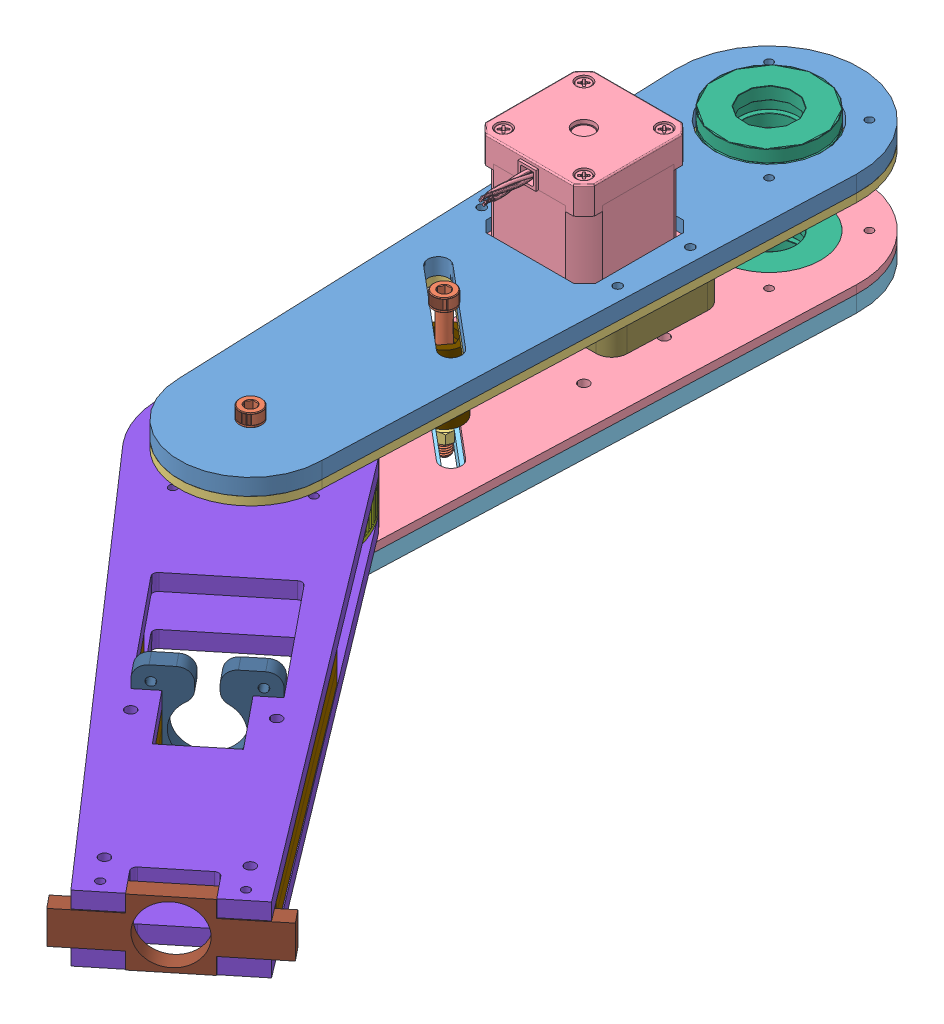
SolidWorks assembly AssemBrasAB, configuration Default. Lengths in mm.
Overall size (236.62 124.43 442.17).
121 component instances, 22 part files, 30 mates.
Components (placement in the parent):
- 03_02_AssemUpperAndLowerArm-1: 03_02_AssemUpperAndLowerArm [Default] at (4.2942 33.9 -117.8774) size (70 11.12 262.5)
  - 03_07_upper&lowerArm-1: 03_07_upper&lowerArm [Default] at (53.4457 141.3704 413.2602) size (70 6.35 262.5)
  - ThrustBallBearingUpper-1: ThrustBallBearingUpper [7806K755] at (53.4457 134.3704 413.2602) x (-0.862828 0 -0.505498) z (-0.505498 0 0.862828) size (40 14 40)
  - upper&lowerbearingFit3mmStepperSide-1: upper&lowerbearingFit3mmStepperSide [Default] at (53.4457 138.1954 313.2602) size (70 3.17 262.5)
- 03_03_AssemUpperAndLowerArm_hex_tete-1: 03_03_AssemUpperAndLowerArm_hex_tete [Défaut] at (77.1604 138.7226 -64.6172) size (70 11.12 262.5)
  - upper&lowerbearingFit3mm-1: upper&lowerbearingFit3mm [Default] at (-19.4206 2.7978 260) size (70 3.17 262.5)
  - 03_07_upper&lowerArm_modif_tete-1: 03_07_upper&lowerArm_modif_tete [Default] at (-19.4206 -3.5522 360) size (70 6.35 262.5)
  - ThrustBallBearingUpper-1: ThrustBallBearingUpper [7806K755] at (-19.4206 9.7978 360) size (40 14 40)
- 03_01_AssemMidArm-1: 03_01_AssemMidArm [Default] at (-73.2329 23.0648 -64.757) x (0.817633 0.030604 -0.574926) z (0.569769 -0.186456 0.800374) size (99.53 73.91 261.74)
  - 7806K755_Thrust Ball Bearing-6: 7806K755_Thrust Ball Bearing [7806K755] at (-95.5251 214.5077 335.8148) x (0.999339 -0.026395 0.025015) z (-0.019643 0.187098 0.982145) size (40 14 40)
  - 7806K755_Thrust Ball Bearing-7: 7806K755_Thrust Ball Bearing [7806K755] at (-96.1234 195.3099 339.46) x (0.408436 -0.182544 -0.894347) z (-0.912274 -0.048784 -0.406666) size (40 14 40)
  - 03_17_customPoulieDenteFinalReworkJoint2-1: 03_17_customPoulieDenteFinalReworkJoint2 [Výchozí] at (-95.8242 204.9088 337.6374) x (-0.644614 0.161957 0.747157) z (0.763896 0.097326 0.637959) size (70 12.55 70)
  - 03_14_BottomArm-2: 03_14_BottomArm [Default] at (-95.535 214.1886 335.8754) x (0.997092 -0.04302 -0.062907) z (0.069795 0.183988 0.980447) size (70 6.35 246.35)
  - 03_04_midArmUpper-3: 03_04_midArmUpper [Default] at (-95.7196 207.9788 337.1973) x (0.997092 -0.04302 -0.062907) z (0.069795 0.183988 0.980447) size (64 6.35 119.86)
  - 03_15_SupportStepper-1: 03_15_SupportStepper [Default] at (-88.2433 224.8255 444.177) x (0.997092 -0.04302 -0.062907) z (0.069795 0.183988 0.980447) size (57.3 42 6.35)
  - 03_04_midArmUpper-4: 03_04_midArmUpper [Default] at (-95.9139 201.7432 338.3813) x (0.997092 -0.04302 -0.062907) z (0.069795 0.183988 0.980447) size (64 6.35 119.86)
  - 03_14_BottomArm-3: 03_14_BottomArm [Default] at (-96.1181 195.4817 339.4274) x (0.997092 -0.04302 -0.062907) z (0.069795 0.183988 0.980447) size (70 6.35 246.35)
  - bearing_holder-1: bearing_holder [Default] at (-81.4941 242.6171 538.9862) x (0.997092 -0.04302 -0.062907) z (-0.030604 -0.981987 0.186456) size (68.18 6.35 25.4)
- 7806K755_Thrust Ball Bearing-1: 7806K755_Thrust Ball Bearing [7806K755] at (57.7399 137.6954 95.3828) x (0.884024 0 -0.467442) z (-0.467442 0 -0.884024) size (40 14 40)
- 7806K755_Thrust Ball Bearing-2: 7806K755_Thrust Ball Bearing [7806K755] at (57.7399 178.9954 95.3828) x (0.977918 0 -0.208988) z (0.208988 0 0.977918) size (40 14 40)
- 03_016_supportStepper-1: 03_016_supportStepper [Default] at (57.5899 162.5204 166.6828) x (0 0 1) z (-1 0 0) size (42 9.57 65.8)
- T5 Pulley-1: T5 Pulley [Predeterminado] at (58.5899 147.6204 166.6828) x (0 1 0) z (0.997679 0 0.068096) size (14.8 16 16)
- Bearing Subassy, GT2 Idler Pulley, Configurable-1: Bearing Subassy, GT2 Idler Pulley, Configurable [5 mm Bore] at (58.5899 143.0204 166.6828) size (9 3 9)
  - Bearing Outer Ring, GT2 Idler Pulley, Configurable-1: Bearing Outer Ring, GT2 Idler Pulley, Configurable [5 mm Bore] at origin size (9 3 9)
  - Bearing Inner Ring, GT2 Idler Pulley, Configurable-1: Bearing Inner Ring, GT2 Idler Pulley, Configurable [5 mm Bore] x (0.926062 0 -0.377371) z (0.377371 0 0.926062) size (6 3 6)
  - Bearing Seal, GT2 Idler Pulley, Configurable-1: Bearing Seal, GT2 Idler Pulley, Configurable [5 mm Bore] at (0 1.25 0) size (8 0.5 8)
  - Bearing Seal, GT2 Idler Pulley, Configurable-2: Bearing Seal, GT2 Idler Pulley, Configurable [5 mm Bore] at (0 -1.25 0) x (1 0 0) z (0 0 -1) size (8 0.5 8)
  - Bearing Ball, GT2 Idler Pulley, Configurable-1: Bearing Ball, GT2 Idler Pulley, Configurable [1.4 mm] at (-2.4745 0 -2.4753) x (-0.715461 0 0.698652) z (-0.698652 0 -0.715461) size (1.4 1.4 1.4)
  - Bearing Ball, GT2 Idler Pulley, Configurable-2: Bearing Ball, GT2 Idler Pulley, Configurable [1.4 mm] at (-0.9053 0 -3.3809) x (-0.968934 0 0.24732) z (-0.24732 0 -0.968934) size (1.4 1.4 1.4)
  - Bearing Ball, GT2 Idler Pulley, Configurable-3: Bearing Ball, GT2 Idler Pulley, Configurable [1.4 mm] at (0.9064 0 -3.3806) x (-0.962781 0 -0.270282) z (0.270282 0 -0.962781) size (1.4 1.4 1.4)
  - Bearing Ball, GT2 Idler Pulley, Configurable-4: Bearing Ball, GT2 Idler Pulley, Configurable [1.4 mm] at (2.4753 0 -2.4745) x (-0.698652 0 -0.715461) z (0.715461 0 -0.698652) size (1.4 1.4 1.4)
  - Bearing Ball, GT2 Idler Pulley, Configurable-5: Bearing Ball, GT2 Idler Pulley, Configurable [1.4 mm] at (3.3809 0 -0.9053) x (-0.24732 0 -0.968934) z (0.968934 0 -0.24732) size (1.4 1.4 1.4)
  - Bearing Ball, GT2 Idler Pulley, Configurable-6: Bearing Ball, GT2 Idler Pulley, Configurable [1.4 mm] at (3.3806 0 0.9064) x (0.270282 0 -0.962781) z (0.962781 0 0.270282) size (1.4 1.4 1.4)
  - Bearing Ball, GT2 Idler Pulley, Configurable-7: Bearing Ball, GT2 Idler Pulley, Configurable [1.4 mm] at (2.4745 0 2.4753) x (0.715461 0 -0.698652) z (0.698652 0 0.715461) size (1.4 1.4 1.4)
  - Bearing Ball, GT2 Idler Pulley, Configurable-8: Bearing Ball, GT2 Idler Pulley, Configurable [1.4 mm] at (0.9053 0 3.3809) x (0.968934 0 -0.24732) z (0.24732 0 0.968934) size (1.4 1.4 1.4)
  - Bearing Ball, GT2 Idler Pulley, Configurable-9: Bearing Ball, GT2 Idler Pulley, Configurable [1.4 mm] at (-0.9064 0 3.3806) x (0.962781 0 0.270282) z (-0.270282 0 0.962781) size (1.4 1.4 1.4)
  - Bearing Ball, GT2 Idler Pulley, Configurable-10: Bearing Ball, GT2 Idler Pulley, Configurable [1.4 mm] at (-2.4753 0 2.4745) x (0.698652 0 0.715461) z (-0.715461 0 0.698652) size (1.4 1.4 1.4)
  - Bearing Ball, GT2 Idler Pulley, Configurable-11: Bearing Ball, GT2 Idler Pulley, Configurable [1.4 mm] at (-3.3809 0 0.9053) x (0.24732 0 0.968934) z (-0.968934 0 0.24732) size (1.4 1.4 1.4)
  - Bearing Ball, GT2 Idler Pulley, Configurable-12: Bearing Ball, GT2 Idler Pulley, Configurable [1.4 mm] at (-3.3806 0 -0.9064) x (-0.270282 0 0.962781) z (-0.962781 0 -0.270282) size (1.4 1.4 1.4)
- pulleyColonne-1: pulleyColonne [Default] at (56.6305 171.1954 219.6076) x (-0.741677 0 -0.670758) z (-0.670758 0 0.741677) size (20 9 20)
- pulleyColonne-2: pulleyColonne [Default] at (56.6305 144.6954 219.6076) size (20 9 20)
- GT2 Idler Pulley, Configurable-1: GT2 Idler Pulley, Configurable [20T W6 B5 Without T] at (56.6305 157.9454 219.6076) x (-0.778121 0 0.628114) z (-0.628114 0 -0.778121) size (25.32 8.5 25.32)
  - Body, GT2 Idler Pulley, Configurable-1: Body, GT2 Idler Pulley, Configurable [20T W6 B5 Without T] x (-0.63029 0 -0.77636) z (0.77636 0 -0.63029) size (18 8.5 18)
  - Bearing Subassy, GT2 Idler Pulley, Configurable-1: Bearing Subassy, GT2 Idler Pulley, Configurable [5 mm Bore] at (0 2.75 0) x (0.63029 0 0.77636) z (-0.77636 0 0.63029) size (9 3 9)
    - Bearing Outer Ring, GT2 Idler Pulley, Configurable-1: Bearing Outer Ring, GT2 Idler Pulley, Configurable [5 mm Bore] at origin size (9 3 9)
    - Bearing Inner Ring, GT2 Idler Pulley, Configurable-1: Bearing Inner Ring, GT2 Idler Pulley, Configurable [5 mm Bore] x (0.926062 0 -0.377371) z (0.377371 0 0.926062) size (6 3 6)
    - Bearing Seal, GT2 Idler Pulley, Configurable-1: Bearing Seal, GT2 Idler Pulley, Configurable [5 mm Bore] at (0 1.25 0) size (8 0.5 8)
    - Bearing Seal, GT2 Idler Pulley, Configurable-2: Bearing Seal, GT2 Idler Pulley, Configurable [5 mm Bore] at (0 -1.25 0) x (1 0 0) z (0 0 -1) size (8 0.5 8)
    - Bearing Ball, GT2 Idler Pulley, Configurable-1: Bearing Ball, GT2 Idler Pulley, Configurable [1.4 mm] at (-2.4745 0 -2.4753) x (-0.715461 0 0.698652) z (-0.698652 0 -0.715461) size (1.4 1.4 1.4)
    - Bearing Ball, GT2 Idler Pulley, Configurable-2: Bearing Ball, GT2 Idler Pulley, Configurable [1.4 mm] at (-0.9053 0 -3.3809) x (-0.968934 0 0.24732) z (-0.24732 0 -0.968934) size (1.4 1.4 1.4)
    - Bearing Ball, GT2 Idler Pulley, Configurable-3: Bearing Ball, GT2 Idler Pulley, Configurable [1.4 mm] at (0.9064 0 -3.3806) x (-0.962781 0 -0.270282) z (0.270282 0 -0.962781) size (1.4 1.4 1.4)
    - Bearing Ball, GT2 Idler Pulley, Configurable-4: Bearing Ball, GT2 Idler Pulley, Configurable [1.4 mm] at (2.4753 0 -2.4745) x (-0.698652 0 -0.715461) z (0.715461 0 -0.698652) size (1.4 1.4 1.4)
    - Bearing Ball, GT2 Idler Pulley, Configurable-5: Bearing Ball, GT2 Idler Pulley, Configurable [1.4 mm] at (3.3809 0 -0.9053) x (-0.24732 0 -0.968934) z (0.968934 0 -0.24732) size (1.4 1.4 1.4)
    - Bearing Ball, GT2 Idler Pulley, Configurable-6: Bearing Ball, GT2 Idler Pulley, Configurable [1.4 mm] at (3.3806 0 0.9064) x (0.270282 0 -0.962781) z (0.962781 0 0.270282) size (1.4 1.4 1.4)
    - Bearing Ball, GT2 Idler Pulley, Configurable-7: Bearing Ball, GT2 Idler Pulley, Configurable [1.4 mm] at (2.4745 0 2.4753) x (0.715461 0 -0.698652) z (0.698652 0 0.715461) size (1.4 1.4 1.4)
    - Bearing Ball, GT2 Idler Pulley, Configurable-8: Bearing Ball, GT2 Idler Pulley, Configurable [1.4 mm] at (0.9053 0 3.3809) x (0.968934 0 -0.24732) z (0.24732 0 0.968934) size (1.4 1.4 1.4)
    - Bearing Ball, GT2 Idler Pulley, Configurable-9: Bearing Ball, GT2 Idler Pulley, Configurable [1.4 mm] at (-0.9064 0 3.3806) x (0.962781 0 0.270282) z (-0.270282 0 0.962781) size (1.4 1.4 1.4)
    - Bearing Ball, GT2 Idler Pulley, Configurable-10: Bearing Ball, GT2 Idler Pulley, Configurable [1.4 mm] at (-2.4753 0 2.4745) x (0.698652 0 0.715461) z (-0.715461 0 0.698652) size (1.4 1.4 1.4)
    - Bearing Ball, GT2 Idler Pulley, Configurable-11: Bearing Ball, GT2 Idler Pulley, Configurable [1.4 mm] at (-3.3809 0 0.9053) x (0.24732 0 0.968934) z (-0.968934 0 0.24732) size (1.4 1.4 1.4)
    - Bearing Ball, GT2 Idler Pulley, Configurable-12: Bearing Ball, GT2 Idler Pulley, Configurable [1.4 mm] at (-3.3806 0 -0.9064) x (-0.270282 0 0.962781) z (-0.962781 0 -0.270282) size (1.4 1.4 1.4)
  - Bearing Subassy, GT2 Idler Pulley, Configurable-2: Bearing Subassy, GT2 Idler Pulley, Configurable [5 mm Bore] at (0 -2.75 0) x (0.63029 0 0.77636) z (0.77636 0 -0.63029) size (9 3 9)
    - Bearing Outer Ring, GT2 Idler Pulley, Configurable-1: Bearing Outer Ring, GT2 Idler Pulley, Configurable [5 mm Bore] at origin size (9 3 9)
    - Bearing Inner Ring, GT2 Idler Pulley, Configurable-1: Bearing Inner Ring, GT2 Idler Pulley, Configurable [5 mm Bore] x (0.926062 0 -0.377371) z (0.377371 0 0.926062) size (6 3 6)
    - Bearing Seal, GT2 Idler Pulley, Configurable-1: Bearing Seal, GT2 Idler Pulley, Configurable [5 mm Bore] at (0 1.25 0) size (8 0.5 8)
    - Bearing Seal, GT2 Idler Pulley, Configurable-2: Bearing Seal, GT2 Idler Pulley, Configurable [5 mm Bore] at (0 -1.25 0) x (1 0 0) z (0 0 -1) size (8 0.5 8)
    - Bearing Ball, GT2 Idler Pulley, Configurable-1: Bearing Ball, GT2 Idler Pulley, Configurable [1.4 mm] at (-2.4745 0 -2.4753) x (-0.715461 0 0.698652) z (-0.698652 0 -0.715461) size (1.4 1.4 1.4)
    - Bearing Ball, GT2 Idler Pulley, Configurable-2: Bearing Ball, GT2 Idler Pulley, Configurable [1.4 mm] at (-0.9053 0 -3.3809) x (-0.968934 0 0.24732) z (-0.24732 0 -0.968934) size (1.4 1.4 1.4)
    - Bearing Ball, GT2 Idler Pulley, Configurable-3: Bearing Ball, GT2 Idler Pulley, Configurable [1.4 mm] at (0.9064 0 -3.3806) x (-0.962781 0 -0.270282) z (0.270282 0 -0.962781) size (1.4 1.4 1.4)
    - Bearing Ball, GT2 Idler Pulley, Configurable-4: Bearing Ball, GT2 Idler Pulley, Configurable [1.4 mm] at (2.4753 0 -2.4745) x (-0.698652 0 -0.715461) z (0.715461 0 -0.698652) size (1.4 1.4 1.4)
    - Bearing Ball, GT2 Idler Pulley, Configurable-5: Bearing Ball, GT2 Idler Pulley, Configurable [1.4 mm] at (3.3809 0 -0.9053) x (-0.24732 0 -0.968934) z (0.968934 0 -0.24732) size (1.4 1.4 1.4)
    - Bearing Ball, GT2 Idler Pulley, Configurable-6: Bearing Ball, GT2 Idler Pulley, Configurable [1.4 mm] at (3.3806 0 0.9064) x (0.270282 0 -0.962781) z (0.962781 0 0.270282) size (1.4 1.4 1.4)
    - Bearing Ball, GT2 Idler Pulley, Configurable-7: Bearing Ball, GT2 Idler Pulley, Configurable [1.4 mm] at (2.4745 0 2.4753) x (0.715461 0 -0.698652) z (0.698652 0 0.715461) size (1.4 1.4 1.4)
    - Bearing Ball, GT2 Idler Pulley, Configurable-8: Bearing Ball, GT2 Idler Pulley, Configurable [1.4 mm] at (0.9053 0 3.3809) x (0.968934 0 -0.24732) z (0.24732 0 0.968934) size (1.4 1.4 1.4)
    - Bearing Ball, GT2 Idler Pulley, Configurable-9: Bearing Ball, GT2 Idler Pulley, Configurable [1.4 mm] at (-0.9064 0 3.3806) x (0.962781 0 0.270282) z (-0.270282 0 0.962781) size (1.4 1.4 1.4)
    - Bearing Ball, GT2 Idler Pulley, Configurable-10: Bearing Ball, GT2 Idler Pulley, Configurable [1.4 mm] at (-2.4753 0 2.4745) x (0.698652 0 0.715461) z (-0.715461 0 0.698652) size (1.4 1.4 1.4)
    - Bearing Ball, GT2 Idler Pulley, Configurable-11: Bearing Ball, GT2 Idler Pulley, Configurable [1.4 mm] at (-3.3809 0 0.9053) x (0.24732 0 0.968934) z (-0.968934 0 0.24732) size (1.4 1.4 1.4)
    - Bearing Ball, GT2 Idler Pulley, Configurable-12: Bearing Ball, GT2 Idler Pulley, Configurable [1.4 mm] at (-3.3806 0 -0.9064) x (-0.270282 0 0.962781) z (-0.962781 0 -0.270282) size (1.4 1.4 1.4)
- 91290A262_Black-Oxide Alloy Steel Socket Head Screw-1: 91290A262_Black-Oxide Alloy Steel Socket Head Screw [91290A262] at (56.6305 159.1204 219.6076) x (-0.61715 0 -0.786845) z (0 1 0) size (8.5 8.5 55.38)
- 90592A095_Steel Hex Nut-1: 90592A095_Steel Hex Nut [90592A095] at (56.6305 139.5204 219.6076) x (0.642788 0 -0.766044) z (0.766044 0 0.642788) size (8 4.62 9.24)
- 91290A262_Black-Oxide Alloy Steel Socket Head Screw-2: 91290A262_Black-Oxide Alloy Steel Socket Head Screw [91290A262] at (57.7399 159.1204 295.3828) x (1 0 0) z (0 1 0) size (8.5 8.5 55.38)
- 90592A095_Steel Hex Nut-2: 90592A095_Steel Hex Nut [90592A095] at (57.7399 133.1704 295.3828) x (1 0 0) z (0 0 -1) size (8 4.62 9.24)
- GT2 Idler Pulley, Configurable-2: GT2 Idler Pulley, Configurable [20T W6 B5 Without T] at (65.7399 157.9454 202.6394) x (-0.990708 0 -0.136005) z (0.136005 0 -0.990708) size (25.32 8.5 25.32) (suppressed, hidden)
  - Body, GT2 Idler Pulley, Configurable-1: Body, GT2 Idler Pulley, Configurable [20T W6 B5 Without T] x (-0.63029 0 -0.77636) z (0.77636 0 -0.63029) size (18 8.5 18)
  - Bearing Subassy, GT2 Idler Pulley, Configurable-1: Bearing Subassy, GT2 Idler Pulley, Configurable [5 mm Bore] at (0 2.75 0) x (0.63029 0 0.77636) z (-0.77636 0 0.63029) size (9 3 9)
    - Bearing Outer Ring, GT2 Idler Pulley, Configurable-1: Bearing Outer Ring, GT2 Idler Pulley, Configurable [5 mm Bore] at origin size (9 3 9)
    - Bearing Inner Ring, GT2 Idler Pulley, Configurable-1: Bearing Inner Ring, GT2 Idler Pulley, Configurable [5 mm Bore] x (0.926062 0 -0.377371) z (0.377371 0 0.926062) size (6 3 6)
    - Bearing Seal, GT2 Idler Pulley, Configurable-1: Bearing Seal, GT2 Idler Pulley, Configurable [5 mm Bore] at (0 1.25 0) size (8 0.5 8)
    - Bearing Seal, GT2 Idler Pulley, Configurable-2: Bearing Seal, GT2 Idler Pulley, Configurable [5 mm Bore] at (0 -1.25 0) x (1 0 0) z (0 0 -1) size (8 0.5 8)
    - Bearing Ball, GT2 Idler Pulley, Configurable-1: Bearing Ball, GT2 Idler Pulley, Configurable [1.4 mm] at (-2.4745 0 -2.4753) x (-0.715461 0 0.698652) z (-0.698652 0 -0.715461) size (1.4 1.4 1.4)
    - Bearing Ball, GT2 Idler Pulley, Configurable-2: Bearing Ball, GT2 Idler Pulley, Configurable [1.4 mm] at (-0.9053 0 -3.3809) x (-0.968934 0 0.24732) z (-0.24732 0 -0.968934) size (1.4 1.4 1.4)
    - Bearing Ball, GT2 Idler Pulley, Configurable-3: Bearing Ball, GT2 Idler Pulley, Configurable [1.4 mm] at (0.9064 0 -3.3806) x (-0.962781 0 -0.270282) z (0.270282 0 -0.962781) size (1.4 1.4 1.4)
    - Bearing Ball, GT2 Idler Pulley, Configurable-4: Bearing Ball, GT2 Idler Pulley, Configurable [1.4 mm] at (2.4753 0 -2.4745) x (-0.698652 0 -0.715461) z (0.715461 0 -0.698652) size (1.4 1.4 1.4)
    - Bearing Ball, GT2 Idler Pulley, Configurable-5: Bearing Ball, GT2 Idler Pulley, Configurable [1.4 mm] at (3.3809 0 -0.9053) x (-0.24732 0 -0.968934) z (0.968934 0 -0.24732) size (1.4 1.4 1.4)
    - Bearing Ball, GT2 Idler Pulley, Configurable-6: Bearing Ball, GT2 Idler Pulley, Configurable [1.4 mm] at (3.3806 0 0.9064) x (0.270282 0 -0.962781) z (0.962781 0 0.270282) size (1.4 1.4 1.4)
    - Bearing Ball, GT2 Idler Pulley, Configurable-7: Bearing Ball, GT2 Idler Pulley, Configurable [1.4 mm] at (2.4745 0 2.4753) x (0.715461 0 -0.698652) z (0.698652 0 0.715461) size (1.4 1.4 1.4)
    - Bearing Ball, GT2 Idler Pulley, Configurable-8: Bearing Ball, GT2 Idler Pulley, Configurable [1.4 mm] at (0.9053 0 3.3809) x (0.968934 0 -0.24732) z (0.24732 0 0.968934) size (1.4 1.4 1.4)
    - Bearing Ball, GT2 Idler Pulley, Configurable-9: Bearing Ball, GT2 Idler Pulley, Configurable [1.4 mm] at (-0.9064 0 3.3806) x (0.962781 0 0.270282) z (-0.270282 0 0.962781) size (1.4 1.4 1.4)
    - Bearing Ball, GT2 Idler Pulley, Configurable-10: Bearing Ball, GT2 Idler Pulley, Configurable [1.4 mm] at (-2.4753 0 2.4745) x (0.698652 0 0.715461) z (-0.715461 0 0.698652) size (1.4 1.4 1.4)
    - Bearing Ball, GT2 Idler Pulley, Configurable-11: Bearing Ball, GT2 Idler Pulley, Configurable [1.4 mm] at (-3.3809 0 0.9053) x (0.24732 0 0.968934) z (-0.968934 0 0.24732) size (1.4 1.4 1.4)
    - Bearing Ball, GT2 Idler Pulley, Configurable-12: Bearing Ball, GT2 Idler Pulley, Configurable [1.4 mm] at (-3.3806 0 -0.9064) x (-0.270282 0 0.962781) z (-0.962781 0 -0.270282) size (1.4 1.4 1.4)
  - Bearing Subassy, GT2 Idler Pulley, Configurable-2: Bearing Subassy, GT2 Idler Pulley, Configurable [5 mm Bore] at (0 -2.75 0) x (0.63029 0 0.77636) z (0.77636 0 -0.63029) size (9 3 9)
    - Bearing Outer Ring, GT2 Idler Pulley, Configurable-1: Bearing Outer Ring, GT2 Idler Pulley, Configurable [5 mm Bore] at origin size (9 3 9)
    - Bearing Inner Ring, GT2 Idler Pulley, Configurable-1: Bearing Inner Ring, GT2 Idler Pulley, Configurable [5 mm Bore] x (0.926062 0 -0.377371) z (0.377371 0 0.926062) size (6 3 6)
    - Bearing Seal, GT2 Idler Pulley, Configurable-1: Bearing Seal, GT2 Idler Pulley, Configurable [5 mm Bore] at (0 1.25 0) size (8 0.5 8)
    - Bearing Seal, GT2 Idler Pulley, Configurable-2: Bearing Seal, GT2 Idler Pulley, Configurable [5 mm Bore] at (0 -1.25 0) x (1 0 0) z (0 0 -1) size (8 0.5 8)
    - Bearing Ball, GT2 Idler Pulley, Configurable-1: Bearing Ball, GT2 Idler Pulley, Configurable [1.4 mm] at (-2.4745 0 -2.4753) x (-0.715461 0 0.698652) z (-0.698652 0 -0.715461) size (1.4 1.4 1.4)
    - Bearing Ball, GT2 Idler Pulley, Configurable-2: Bearing Ball, GT2 Idler Pulley, Configurable [1.4 mm] at (-0.9053 0 -3.3809) x (-0.968934 0 0.24732) z (-0.24732 0 -0.968934) size (1.4 1.4 1.4)
    - Bearing Ball, GT2 Idler Pulley, Configurable-3: Bearing Ball, GT2 Idler Pulley, Configurable [1.4 mm] at (0.9064 0 -3.3806) x (-0.962781 0 -0.270282) z (0.270282 0 -0.962781) size (1.4 1.4 1.4)
    - Bearing Ball, GT2 Idler Pulley, Configurable-4: Bearing Ball, GT2 Idler Pulley, Configurable [1.4 mm] at (2.4753 0 -2.4745) x (-0.698652 0 -0.715461) z (0.715461 0 -0.698652) size (1.4 1.4 1.4)
    - Bearing Ball, GT2 Idler Pulley, Configurable-5: Bearing Ball, GT2 Idler Pulley, Configurable [1.4 mm] at (3.3809 0 -0.9053) x (-0.24732 0 -0.968934) z (0.968934 0 -0.24732) size (1.4 1.4 1.4)
    - Bearing Ball, GT2 Idler Pulley, Configurable-6: Bearing Ball, GT2 Idler Pulley, Configurable [1.4 mm] at (3.3806 0 0.9064) x (0.270282 0 -0.962781) z (0.962781 0 0.270282) size (1.4 1.4 1.4)
    - Bearing Ball, GT2 Idler Pulley, Configurable-7: Bearing Ball, GT2 Idler Pulley, Configurable [1.4 mm] at (2.4745 0 2.4753) x (0.715461 0 -0.698652) z (0.698652 0 0.715461) size (1.4 1.4 1.4)
    - Bearing Ball, GT2 Idler Pulley, Configurable-8: Bearing Ball, GT2 Idler Pulley, Configurable [1.4 mm] at (0.9053 0 3.3809) x (0.968934 0 -0.24732) z (0.24732 0 0.968934) size (1.4 1.4 1.4)
    - Bearing Ball, GT2 Idler Pulley, Configurable-9: Bearing Ball, GT2 Idler Pulley, Configurable [1.4 mm] at (-0.9064 0 3.3806) x (0.962781 0 0.270282) z (-0.270282 0 0.962781) size (1.4 1.4 1.4)
    - Bearing Ball, GT2 Idler Pulley, Configurable-10: Bearing Ball, GT2 Idler Pulley, Configurable [1.4 mm] at (-2.4753 0 2.4745) x (0.698652 0 0.715461) z (-0.715461 0 0.698652) size (1.4 1.4 1.4)
    - Bearing Ball, GT2 Idler Pulley, Configurable-11: Bearing Ball, GT2 Idler Pulley, Configurable [1.4 mm] at (-3.3809 0 0.9053) x (0.24732 0 0.968934) z (-0.968934 0 0.24732) size (1.4 1.4 1.4)
    - Bearing Ball, GT2 Idler Pulley, Configurable-12: Bearing Ball, GT2 Idler Pulley, Configurable [1.4 mm] at (-3.3806 0 -0.9064) x (-0.270282 0 0.962781) z (-0.962781 0 -0.270282) size (1.4 1.4 1.4)
- pulleyColonne-3: pulleyColonne [Default] at (65.7399 144.6954 202.6394) x (-1 0 0) z (0 0 -1) size (20 9 20) (suppressed, hidden)
- 91290A262_Black-Oxide Alloy Steel Socket Head Screw-3: 91290A262_Black-Oxide Alloy Steel Socket Head Screw [91290A262] at (65.7399 159.1204 204.422) x (-0.010234 0 -0.999948) z (0 1 0) size (8.5 8.5 55.38) (suppressed, hidden)
- pulleyColonne-4: pulleyColonne [Default] at (65.7399 171.1954 204.422) x (0.741677 0 -0.670758) z (-0.670758 0 -0.741677) size (20 9 20) (suppressed, hidden)
- NEMA17 x 48-1: NEMA17 x 48 [Default] at (57.5899 166.5204 166.6828) size (42 72 60)
Mates (geometry in assembly coordinates):
- Concentric3: concentric anti-aligned: circle of 03_02_AssemUpperAndLowerArm-1/ThrustBallBearingUpper-1; circle of 03_03_AssemUpperAndLowerArm_hex_tete-1/ThrustBallBearingUpper-1
- Concentric5: concentric anti-aligned: circle of 03_03_AssemUpperAndLowerArm_hex_tete-1/ThrustBallBearingUpper-1; circle of 03_01_AssemMidArm-1/7806K755_Thrust Ball Bearing-7
- Concentric7: concentric aligned: circle of 03_03_AssemUpperAndLowerArm_hex_tete-1/03_07_upper&lowerArm_modif_tete-1; circle of 7806K755_Thrust Ball Bearing-1
- Concentric8: concentric anti-aligned: circle of 03_02_AssemUpperAndLowerArm-1/03_07_upper&lowerArm-1; circle of 7806K755_Thrust Ball Bearing-2
- Distance1: distance = 14.1 mm anti-aligned: plane of 03_01_AssemMidArm-1/03_17_customPoulieDenteFinalReworkJoint2-1 through (57.7399 161.1704 295.3828) normal (0 1 0); plane of 03_02_AssemUpperAndLowerArm-1/03_07_upper&lowerArm-1 through (57.7399 175.2704 295.3828) normal (0 -1 0)
- Distance2: distance = 14.1 mm anti-aligned: plane of 03_01_AssemMidArm-1/03_17_customPoulieDenteFinalReworkJoint2-1 through (57.7399 155.6204 295.3828) normal (0 -1 0); plane of 03_03_AssemUpperAndLowerArm_hex_tete-1/03_07_upper&lowerArm_modif_tete-1 through (57.7399 141.5204 295.3828) normal (0 1 0)
- Coincident4: coincident aligned: plane of 03_01_AssemMidArm-1/03_17_customPoulieDenteFinalReworkJoint2-1 through (57.7399 153.6204 295.3828) normal (0 1 0); plane of T5 Pulley-1 through (58.1132 153.6204 173.6665) normal (0 1 0)
- Coincident6: coincident anti-aligned: plane of 03_03_AssemUpperAndLowerArm_hex_tete-1/03_07_upper&lowerArm_modif_tete-1 through (57.7399 141.5204 295.3828) normal (0 1 0); plane of Bearing Subassy, GT2 Idler Pulley, Configurable-1/Bearing Outer Ring, GT2 Idler Pulley, Configurable-1 through (58.5899 141.5204 166.6828) normal (0 -1 0)
- Concentric15: concentric aligned: cylinder of 03_03_AssemUpperAndLowerArm_hex_tete-1/upper&lowerbearingFit3mm-1 through (58.5899 141.5204 166.6828) axis (0 1 0) radius 4.425; circle of Bearing Subassy, GT2 Idler Pulley, Configurable-1/Bearing Outer Ring, GT2 Idler Pulley, Configurable-1
- Coincident22: coincident anti-aligned: plane of pulleyColonne-2 through (56.6305 153.6954 219.6076) normal (0 1 0); plane of GT2 Idler Pulley, Configurable-1/Body, GT2 Idler Pulley, Configurable-1 through (61.0318 153.6954 220.5446) normal (0 -1 0)
- Concentric20: concentric: circle of pulleyColonne-2; circle of GT2 Idler Pulley, Configurable-1/Body, GT2 Idler Pulley, Configurable-1
- Coincident23: coincident anti-aligned: plane of pulleyColonne-1 through (56.6305 162.1954 219.6076) normal (0 -1 0); plane of GT2 Idler Pulley, Configurable-1/Body, GT2 Idler Pulley, Configurable-1 through (65.4332 162.1954 221.4815) normal (0 1 0)
- Coincident24: coincident: plane of 03_03_AssemUpperAndLowerArm_hex_tete-1/upper&lowerbearingFit3mm-1 through (57.7399 144.6954 195.3828) normal (0 1 0); plane of pulleyColonne-2 through (56.6305 144.6954 219.6076) normal (0 -1 0)
- Slot1: slot: cylinder of assembly; plane of assembly; cylinder of pulleyColonne-2 through (56.6305 153.6954 219.6076) axis (0 -1 0) radius 3; plane of 03_03_AssemUpperAndLowerArm_hex_tete-1/03_07_upper&lowerArm_modif_tete-1 through (74.6677 135.1704 231.4792) normal (-0.642788 0 0.766044); cylinder of 03_03_AssemUpperAndLowerArm_hex_tete-1/03_07_upper&lowerArm_modif_tete-1 through (42.419 135.1704 207.6828) axis (0 1 0) radius 2.5
- Coincident25: coincident anti-aligned: plane of 03_02_AssemUpperAndLowerArm-1/03_07_upper&lowerArm-1 through (57.7399 181.6204 295.3828) normal (0 1 0); plane of 91290A262_Black-Oxide Alloy Steel Socket Head Screw-1 through (53.4831 181.6204 222.0762) normal (0 -1 0)
- Concentric22: concentric anti-aligned: cylinder of pulleyColonne-1 through (56.6305 162.1954 219.6076) axis (0 1 0) radius 3; cylinder of 91290A262_Black-Oxide Alloy Steel Socket Head Screw-1 through (56.6305 131.6204 219.6076) axis (0 -1 0) radius 2.5
- Concentric23: concentric: circle of 91290A262_Black-Oxide Alloy Steel Socket Head Screw-1; circle of 90592A095_Steel Hex Nut-1
- Coincident26: coincident: plane of 03_03_AssemUpperAndLowerArm_hex_tete-1/03_07_upper&lowerArm_modif_tete-1 through (74.6677 135.1704 231.4792) normal (-0.642788 0 0.766044); plane of 90592A095_Steel Hex Nut-1 through (60.9707 141.5204 218.0279) normal (0.642788 0 -0.766044)
- Coincident27: coincident anti-aligned: plane of 03_03_AssemUpperAndLowerArm_hex_tete-1/upper&lowerbearingFit3mm-1 through (57.7399 141.5204 195.3828) normal (0 -1 0); plane of 90592A095_Steel Hex Nut-1 through (52.2902 141.5204 221.1874) normal (0 1 0)
- Concentric24: concentric anti-aligned: cylinder of 03_02_AssemUpperAndLowerArm-1/03_07_upper&lowerArm-1 through (57.7399 175.2704 295.3828) axis (0 1 0) radius 2.6; cylinder of 91290A262_Black-Oxide Alloy Steel Socket Head Screw-2 through (57.7399 131.6204 295.3828) axis (0 -1 0) radius 2.5
- Coincident28: coincident anti-aligned: plane of 03_02_AssemUpperAndLowerArm-1/03_07_upper&lowerArm-1 through (57.7399 181.6204 295.3828) normal (0 1 0); plane of 91290A262_Black-Oxide Alloy Steel Socket Head Screw-2 through (57.7399 181.6204 291.3828) normal (0 -1 0)
- Concentric25: concentric aligned: circle of 91290A262_Black-Oxide Alloy Steel Socket Head Screw-2; circle of 90592A095_Steel Hex Nut-2
- Coincident29: coincident anti-aligned: plane of 03_03_AssemUpperAndLowerArm_hex_tete-1/03_07_upper&lowerArm_modif_tete-1 through (57.7399 135.1704 295.3828) normal (0 -1 0); plane of 90592A095_Steel Hex Nut-2 through (53.7399 135.1704 297.6922) normal (0 1 0)
- Parallel3: parallel aligned: plane of 03_02_AssemUpperAndLowerArm-1/03_07_upper&lowerArm-1 through (85.201 181.6204 296.416) normal (0.999293 0 0.037597); plane of 03_03_AssemUpperAndLowerArm_hex_tete-1/03_07_upper&lowerArm_modif_tete-1 through (85.201 141.5204 296.416) normal (0.999293 0 0.037597)
- Concentric27: concentric: cylinder of GT2 Idler Pulley, Configurable-1/Bearing Subassy, GT2 Idler Pulley, Configurable-1/Bearing Inner Ring, GT2 Idler Pulley, Configurable-1 through (56.6305 162.1954 219.6076) axis (0 -1 0) radius 2.5; cylinder of 91290A262_Black-Oxide Alloy Steel Socket Head Screw-1 through (56.6305 131.6204 219.6076) axis (0 -1 0) radius 2.5
- Coincident35: coincident anti-aligned: plane of 03_02_AssemUpperAndLowerArm-1/03_07_upper&lowerArm-1 through (74.7179 175.2704 187.6828) normal (0 0 -1); plane of NEMA17 x 48-1 through (74.5604 214.5204 187.6828) normal (0 0 1)
- Coincident38: coincident anti-aligned: plane of 03_02_AssemUpperAndLowerArm-1/03_07_upper&lowerArm-1 through (36.5899 175.2704 183.5109) normal (1 0 0); plane of NEMA17 x 48-1 through (36.5899 177.0204 183.6534) normal (-1 0 0)
- Concentric28: concentric anti-aligned: circle of 03_016_supportStepper-1; circle of NEMA17 x 48-1
- Parallel4: parallel aligned: plane of 03_016_supportStepper-1 through (79.5899 172.0954 187.6828) normal (-1 0 0); plane of NEMA17 x 48-1 through (36.5899 177.0204 183.6534) normal (-1 0 0)
- Coincident39: coincident anti-aligned: plane of 03_02_AssemUpperAndLowerArm-1/upper&lowerbearingFit3mmStepperSide-1 through (57.7399 172.0954 195.3828) normal (0 -1 0); plane of 03_016_supportStepper-1 through (57.5899 172.0954 166.6828) normal (0 1 0)
